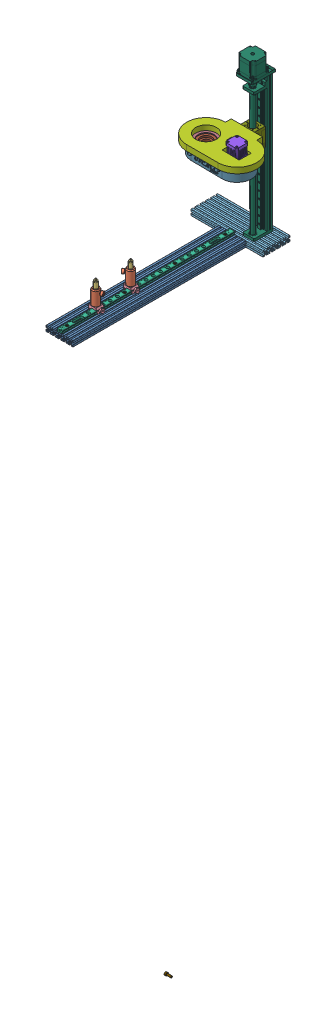
SolidWorks assembly OpenCALAssembly.v3.2, configuration Default. Lengths in mm.
Overall size (733.87 2470.14 969.59).
44 component instances, 19 part files, 57 mates.
Components (placement in the parent):
- 20-2020-Black-25-CL.stp-1: 20-2020-Black-25-CL.stp [Default] at (5.4558 13.0651 39.4201) size (94 20 600)
- PH50_M-Solidworks-1: PH50_M-Solidworks [Default] at (39.4918 57.7304 -95.7663) x (-0.331511 0 -0.943451) z (0.943451 0 -0.331511) size (25 50.44 35.14)
- TR75_M-Solidworks-1: TR75_M-Solidworks [Default] at (34.6119 36.3776 -93.7876) x (0.8365 0 0.547967) z (-0.547967 0 0.8365) size (12.67 80.02 12.87)
- RC1-Solidworks-1: RC1-Solidworks [Default] at (53.5095 23.0651 -81.0876) x (0 0 -1) z (1 0 0) size (25.4 16.53 39.23)
- 20-2020-Black-25-CLShort.stp-1: 20-2020-Black-25-CLShort.stp [Default] at (148.2574 13.0651 -570.5799) x (0 0 -1) z (1 0 0) size (94 20 250)
- PH50_M-Solidworks-2: PH50_M-Solidworks [Default] at (30.7203 57.7304 -211.3859) x (0.637938 0 0.770088) z (-0.770088 0 0.637938) size (25 50.44 35.14)
- TR75_M-Solidworks-2: TR75_M-Solidworks [Default] at (34.6119 34.7631 -214.9333) x (0.31409 0 0.949393) z (-0.949393 0 0.31409) size (12.67 80.02 12.87)
- RC1-Solidworks-2: RC1-Solidworks [Default] at (53.5095 23.0651 -202.2333) x (0 0 -1) z (1 0 0) size (25.4 16.53 39.23)
- RLA600_M-Solidworks-1: RLA600_M-Solidworks [Default] at (42.6639 28.1451 -260.6859) size (19.05 9.53 600)
- OpenCAL Assembly v3.2-1: OpenCAL Assembly v3.2 [Default] at (166.2971 1597.2966 -1408.9239) x (0.015214 0.027547 -0.999505) z (-0.999013 0.042148 -0.014045) size (158.86 120.73 246.6)
  - RotationStage-1: RotationStage [Default] at (-945.6056 1214.5248 22.5457) x (0.99962 0.027547 -0.000581) z (-0.000581 0.042148 0.999111) size (156.58 80 243.35)
  - Stepper with GT2 Pulley and Closed-Loop Belt-1: Stepper with GT2 Pulley and Closed-Loop Belt [Default] at (-980.4903 1273.0893 61.9746) x (-0.000908 0.042139 0.999111) z (0.99962 0.02756 -0.000254) size (166.51 64.5 74)
    - Copy of Assem2^Stepper with GT2 Pulley and Closed-Loop Belt-1: Copy of Assem2^Stepper with GT2 Pulley and Closed-Loop Belt [Default] at origin size (47.8 64.5 42.3) (virtual)
      - Nema17-1: Nema17 [Predeterminado] at (-104.7481 84.323 13.4322) x (0 0 1) z (1 0 0) size (42.3 64.5 47.8)
      - T5 Pulley-1: T5 Pulley [Predeterminado] at (-104.7481 37.623 13.4322) x (0 -1 0) z (0 0 1) size (14.8 16 16)
    - Belt-1: Belt [Default] at (-108.6865 25.623 13.493) size (153.36 6 74)
  - Collet with Gear and Toolholder-1: Collet with Gear and Toolholder [Default] at (-963.7475 1278.8086 52.0713) x (-0.99962 -0.027564 0.000171) z (-0.000991 0.042137 0.999111) size (98.27 60.66 98.27)
    - er32 x 34ths ToolHolderOpenCAL-1: er32 x 34ths ToolHolderOpenCAL [Default] at (-15.7823 32.6902 -13.7293) x (0.420729 0 0.907186) z (0.907186 0 -0.420729) size (74 44.7 74)
    - ER32 COLLET NUT-1: ER32 COLLET NUT [Default] at (3.8533 13.4515 11.5736) x (0 -1 0) z (0.99027 0 0.13916) size (22.61 50 50) (hidden)
    - ER32-20.step-1: ER32-20.step [Default] at (3.6132 -14.2638 13.2822) x (0.698361 0 0.715746) z (0 -1 0) size (32.96 32.96 40.01)
    - BallBearing-1: BallBearing [Default] at (3.6132 11.6902 13.2822) x (0.999353 0 0.035955) z (-0.035955 0 0.999353) size (72 9 72)
    - BallBearing-2: BallBearing [Default] at (3.6132 46.3902 13.2822) x (-0.871455 0 -0.490475) z (-0.490475 0 0.871455) size (72 9 72)
  - Rotation Stage Bottom Plate-1: Rotation Stage Bottom Plate [Default] at (-966.1754 1235.8663 67.174) x (0.00324 -0.042075 -0.999109) z (0.999615 0.027659 0.002077) size (210.36 36.77 134.78)
- ZStageAssm-2: ZStageAssm [Default] at (487.3353 488.304 -911.4771) x (0 -1 0) z (-1 0 0) size (562.65 93.47 86.84)
  - FSL40E350-BC-B57-1: FSL40E350-BC-B57 [Default] at (78.5613 293.4958 501.3397) size (562.65 93.47 86.84)
  - ZCarriage-1: ZCarriage [Default] at (-181.088 293.4958 501.3397) size (67.97 49.14 48.01)
- T-Nut 20 M5 v1.step-1: T-Nut 20 M5 v1.step [Default] at (42.6639 23.0651 14.3141) x (0 0 1) z (-1 0 0) size (10 4.5 9.24)
- socket head cap screw_am1-19: socket head cap screw_am1 [B18.3.1M - 5 x 0.8 x 8 Hex SHCS -- 8NHX] at (42.6639 30.6051 14.3141) x (0 -1 0) z (0 0 1) size (13 8.5 8.5)
- socket head cap screw_am1-20: socket head cap screw_am1 [B18.3.1M - 5 x 0.8 x 8 Hex SHCS -- 8NHX] at (42.6639 30.6051 -535.6859) x (0 -1 0) z (0 0 1) size (13 8.5 8.5)
- socket head cap screw_am1-21: socket head cap screw_am1 [B18.3.1M - 5 x 0.8 x 8 Hex SHCS -- 8NHX] at (42.6639 30.6051 -360.6859) x (0 -1 0) z (0 0 1) size (13 8.5 8.5)
- socket head cap screw_am1-22: socket head cap screw_am1 [B18.3.1M - 5 x 0.8 x 8 Hex SHCS -- 8NHX] at (42.6639 30.6051 -185.6859) x (0 -1 0) z (0 0 1) size (13 8.5 8.5)
- socket head cap screw_am1-23: socket head cap screw_am1 [B18.3.1M - 3 x 0.5 x 10 Hex SHCS -- 10NHX] at (156.5338 336.2143 -461.8522) x (0 1 0) z (0 0 1) size (13 5.5 5.5)
- socket head cap screw_am1-24: socket head cap screw_am1 [B18.3.1M - 3 x 0.5 x 10 Hex SHCS -- 10NHX] at (156.9774 336.2143 -492.8491) x (0 1 0) z (0 0 1) size (13 5.5 5.5)
- socket head cap screw_am1-25: socket head cap screw_am1 [B18.3.1M - 3 x 0.5 x 10 Hex SHCS -- 10NHX] at (125.9806 336.2143 -493.2927) x (0 1 0) z (0 0 1) size (13 5.5 5.5)
- socket head cap screw_am1-26: socket head cap screw_am1 [B18.3.1M - 3 x 0.5 x 10 Hex SHCS -- 10NHX] at (125.5369 336.2143 -462.2959) x (0 1 0) z (0 0 1) size (13 5.5 5.5)
- socket head cap screw_am1-27: socket head cap screw_am1 [B18.3.1M - 6 x 1.0 x 20 Hex SHCS -- 20NHX] at (97.1413 316.7143 -546.4733) x (0 0 -1) z (1 0 0) size (26 10 10)
- socket head cap screw_am1-28: socket head cap screw_am1 [B18.3.1M - 6 x 1.0 x 20 Hex SHCS -- 20NHX] at (77.1413 316.7143 -546.4733) x (0 0 -1) z (1 0 0) size (26 10 10)
- socket head cap screw_am1-29: socket head cap screw_am1 [B18.3.1M - 6 x 1.0 x 20 Hex SHCS -- 20NHX] at (97.1413 331.7143 -546.4733) x (0 0 -1) z (1 0 0) size (26 10 10)
- socket head cap screw_am1-30: socket head cap screw_am1 [B18.3.1M - 6 x 1.0 x 20 Hex SHCS -- 20NHX] at (77.1413 331.7143 -546.4733) x (0 0 -1) z (1 0 0) size (26 10 10)
- socket head cap screw_am1-31: socket head cap screw_am1 [B18.3.1M - 6 x 1.0 x 16 Hex SHCS -- 16NHX] at (316.7296 -1814.5075 -53.5357) size (22 10 10)
- socket head cap screw_am1-32: socket head cap screw_am1 [B18.3.1M - 6 x 1.0 x 16 Hex SHCS -- 16NHX] at (135.3565 328.2143 -537.5447) x (0 1 0) z (0 0 1) size (22 10 10)
- socket head cap screw_am1-33: socket head cap screw_am1 [B18.3.1M - 6 x 1.0 x 16 Hex SHCS -- 16NHX] at (37.4816 328.2143 -420.4078) x (0 1 0) z (0 0 1) size (22 10 10)
- socket head cap screw_am1-34: socket head cap screw_am1 [B18.3.1M - 6 x 1.0 x 16 Hex SHCS -- 16NHX] at (38.9942 328.2143 -537.4009) x (0 1 0) z (0 0 1) size (22 10 10)
- socket head cap screw_am1-35: socket head cap screw_am1 [B18.3.1M - 6 x 1.0 x 16 Hex SHCS -- 16NHX] at (135.4097 328.2143 -420.3812) x (0 1 0) z (0 0 1) size (22 10 10)
Mates (geometry in assembly coordinates):
- Concentric1: concentric aligned: circle of PH50_M-Solidworks-1; cylinder of TR75_M-Solidworks-1 through (34.6119 111.3838 -93.7876) axis (0 1 0) radius 6.3373
- Concentric2: concentric anti-aligned: circle of PH50_M-Solidworks-1; circle of RC1-Solidworks-1
- Coincident4: coincident anti-aligned: plane of PH50_M-Solidworks-1 through (43.7754 38.5591 -67.7092) normal (0 -1 0); plane of RC1-Solidworks-1 through (21.9119 38.5591 -81.0876) normal (0 1 0)
- Parallel1: parallel aligned: plane of 20-2020-Black-25-CL.stp-1 through (-3.0442 4.5651 39.4201) normal (0 0 1); plane of RC1-Solidworks-1 through (21.9119 23.0651 -81.0876) normal (0 0 1)
- Coincident6: coincident aligned: line of 20-2020-Black-25-CL.stp-1 through (45.5938 23.0651 -560.5799) axis (0 0 1); line of RC1-Solidworks-1 through (45.5938 23.0651 -106.4876) axis (0 0 1)
- Coincident7: coincident anti-aligned: plane of 20-2020-Black-25-CL.stp-1 through (32.4558 23.0651 14.4201) normal (0 1 0); plane of RC1-Solidworks-1 through (21.9119 23.0651 -81.0876) normal (0 -1 0)
- Coincident13: coincident anti-aligned: plane of 20-2020-Black-25-CL.stp-1 through (89.4558 4.5651 14.4201) normal (1 0 0); plane of 20-2020-Black-25-CL.stp-3 through (89.4558 13.0651 -350.9237) normal (-1 0 0)
- Concentric3: concentric aligned: circle of PH50_M-Solidworks-2; cylinder of TR75_M-Solidworks-2 through (34.6119 109.7693 -214.9333) axis (0 1 0) radius 6.3373
- Concentric4: concentric anti-aligned: circle of PH50_M-Solidworks-2; circle of RC1-Solidworks-2
- Coincident21: coincident anti-aligned: plane of PH50_M-Solidworks-2 through (16.9784 38.5591 -236.2196) normal (0 -1 0); plane of RC1-Solidworks-2 through (21.9119 38.5591 -202.2333) normal (0 1 0)
- Parallel2: parallel aligned: plane of 20-2020-Black-25-CL.stp-1 through (-3.0442 4.5651 39.4201) normal (0 0 1); plane of RC1-Solidworks-2 through (21.9119 23.0651 -202.2333) normal (0 0 1)
- Coincident22: coincident aligned: line of 20-2020-Black-25-CL.stp-1 through (45.5938 23.0651 -560.5799) axis (0 0 1); line of RC1-Solidworks-2 through (45.5938 23.0651 -227.6333) axis (0 0 1)
- Coincident23: coincident anti-aligned: plane of 20-2020-Black-25-CL.stp-1 through (32.4558 23.0651 14.4201) normal (0 1 0); plane of RC1-Solidworks-2 through (21.9119 23.0651 -202.2333) normal (0 -1 0)
- Parallel4: parallel anti-aligned: line of 20-2020-Black-25-CL.stp-1 through (50.9558 23.0651 39.4201) axis (-1 0 0); line of RLA600_M-Solidworks-1 through (36.3393 23.3191 39.3141) axis (1 0 0)
- Coincident28: coincident anti-aligned: plane of 20-2020-Black-25-CL.stp-1 through (50.9558 23.0651 14.4201) normal (0 1 0); plane of RLA600_M-Solidworks-1 through (52.1889 23.0651 39.3141) normal (0 -1 0)
- Coincident34: coincident aligned: plane of 20-2020-Black-25-CL.stp-1 through (57.8178 23.0651 14.4201) normal (0 1 0); plane of 20-2020-Black-25-CLShort.stp-1 through (123.2574 23.0651 -567.4419) normal (0 1 0)
- Coincident35: coincident anti-aligned: plane of 20-2020-Black-25-CL.stp-1 through (5.4558 13.0651 -560.5799) normal (0 0 -1); plane of 20-2020-Black-25-CLShort.stp-1 through (123.2574 21.5651 -560.5799) normal (0 0 1)
- Coincident36: coincident anti-aligned: plane of 20-2020-Black-25-CLShort.stp-1 through (123.2574 23.0651 -641.4419) normal (0 1 0); plane of ZStageAssm-2/FSL40E350-BC-B57-1 through (87.1413 23.0651 -604.1733) normal (0 -1 0)
- Parallel5: parallel aligned: plane of 20-2020-Black-25-CLShort.stp-1 through (148.2574 4.5651 -562.0799) normal (1 0 0); plane of ZStageAssm-2/FSL40E350-BC-B57-1 through (107.1413 23.0651 -636.6733) normal (1 0 0)
- Concentric13: concentric anti-aligned: circle of OpenCAL Assembly v3.2-1/RotationStage-1; cylinder of ZStageAssm-2/ZCarriage-1 through (97.1413 316.7143 -566.4733) axis (0 0 1) radius 3
- Parallel8: parallel anti-aligned: plane of OpenCAL Assembly v3.2-1/RotationStage-1 through (141.2662 359.2143 -566.4733) normal (1 0 0); plane of ZStageAssm-2/ZCarriage-1 through (111.1412 291.7143 -586.5733) normal (-1 0 0)
- Coincident42: coincident aligned: plane of OpenCAL Assembly v3.2-1/RotationStage-1 through (78.6927 359.2143 -566.4733) normal (0 0 -1); plane of ZStageAssm-2/ZCarriage-1 through (111.1413 356.7143 -566.4733) normal (0 0 -1)
- Concentric14: concentric aligned: cylinder of OpenCAL Assembly v3.2-1/Rotation Stage Bottom Plate-1 through (135.3565 329.2143 -537.5447) axis (0 -1 0) radius 2.9; cylinder of socket head cap screw_am-3 through (135.3565 296.4643 -537.5447) axis (0 -1 0) radius 5
- Coincident43: coincident anti-aligned: plane of OpenCAL Assembly v3.2-1/Rotation Stage Bottom Plate-1 through (133.3356 334.2143 -539.6246) normal (0 -1 0); plane of socket head cap screw_am-3 through (130.3565 334.2143 -537.5447) normal (0 1 0)
- Concentric15: concentric aligned: cylinder of OpenCAL Assembly v3.2-1/Rotation Stage Bottom Plate-1 through (37.4816 329.2143 -420.4078) axis (0 -1 0) radius 5; cylinder of socket head cap screw_am-4 through (37.4816 296.4643 -420.4078) axis (0 -1 0) radius 5
- Coincident44: coincident anti-aligned: plane of OpenCAL Assembly v3.2-1/Rotation Stage Bottom Plate-1 through (35.4607 334.2143 -422.4877) normal (0 -1 0); plane of socket head cap screw_am-4 through (32.4816 334.2143 -420.4078) normal (0 1 0)
- Concentric16: concentric aligned: cylinder of OpenCAL Assembly v3.2-1/Rotation Stage Bottom Plate-1 through (38.9942 329.2143 -537.4009) axis (0 -1 0) radius 2.9; cylinder of socket head cap screw_am-5 through (38.9942 296.4643 -537.4009) axis (0 -1 0) radius 5
- Coincident45: coincident anti-aligned: plane of OpenCAL Assembly v3.2-1/Rotation Stage Bottom Plate-1 through (36.9733 334.2143 -539.4808) normal (0 -1 0); plane of socket head cap screw_am-5 through (33.9942 334.2143 -537.4009) normal (0 1 0)
- Concentric17: concentric: cylinder of OpenCAL Assembly v3.2-1/Rotation Stage Bottom Plate-1 through (135.4097 329.2143 -420.3812) axis (0 -1 0) radius 2.9; cylinder of socket head cap screw_am-6 through (135.4097 296.4643 -420.3812) axis (0 -1 0) radius 5
- Coincident46: coincident: plane of OpenCAL Assembly v3.2-1/Rotation Stage Bottom Plate-1 through (135.4147 334.2143 -423.2812) normal (0 -1 0); plane of socket head cap screw_am-6 through (130.4097 334.2143 -420.3812) normal (0 1 0)
- Concentric22: concentric aligned: cylinder of OpenCAL Assembly v3.2-1/RotationStage-1 through (97.1413 316.7143 -546.4733) axis (0 0 1) radius 5.5; cylinder of socket head cap screw_am-11 through (97.1413 316.7143 -514.7233) axis (0 0 1) radius 5
- Coincident51: coincident anti-aligned: plane of OpenCAL Assembly v3.2-1/RotationStage-1 through (94.5651 314.3451 -552.4733) normal (0 0 1); plane of socket head cap screw_am-11 through (97.1413 321.7143 -552.4733) normal (0 0 -1)
- Concentric23: concentric aligned: cylinder of OpenCAL Assembly v3.2-1/RotationStage-1 through (77.1413 316.7143 -546.4733) axis (0 0 1) radius 3.5; cylinder of socket head cap screw_am-12 through (77.1413 316.7143 -514.7233) axis (0 0 1) radius 5
- Coincident52: coincident anti-aligned: plane of OpenCAL Assembly v3.2-1/RotationStage-1 through (74.5651 314.3451 -552.4733) normal (0 0 1); plane of socket head cap screw_am-12 through (77.1413 321.7143 -552.4733) normal (0 0 -1)
- Concentric24: concentric aligned: cylinder of OpenCAL Assembly v3.2-1/RotationStage-1 through (97.1413 331.7143 -546.4733) axis (0 0 1) radius 3.5; cylinder of socket head cap screw_am-13 through (97.1413 331.7143 -514.7233) axis (0 0 1) radius 5
- Coincident53: coincident anti-aligned: plane of OpenCAL Assembly v3.2-1/RotationStage-1 through (94.5651 329.3451 -552.4733) normal (0 0 1); plane of socket head cap screw_am-13 through (97.1413 336.7143 -552.4733) normal (0 0 -1)
- Concentric25: concentric aligned: cylinder of OpenCAL Assembly v3.2-1/RotationStage-1 through (77.1413 331.7143 -546.4733) axis (0 0 1) radius 3.5; cylinder of socket head cap screw_am-14 through (77.1413 331.7143 -514.7233) axis (0 0 1) radius 5
- Coincident54: coincident anti-aligned: plane of OpenCAL Assembly v3.2-1/RotationStage-1 through (74.5651 329.3451 -552.4733) normal (0 0 1); plane of socket head cap screw_am-14 through (77.1413 336.7143 -552.4733) normal (0 0 -1)
- Concentric26: concentric anti-aligned: cylinder of OpenCAL Assembly v3.2-1/Stepper with GT2 Pulley and Closed-Loop Belt-1/Copy of Assem2^Stepper with GT2 Pulley and Closed-Loop Belt-1/Nema17-1 through (156.5338 388.748 -461.8522) axis (0 1 0) radius 1.6; cylinder of socket head cap screw_am-15 through (156.5338 304.4643 -461.8522) axis (0 -1 0) radius 2.75
- Coincident55: coincident anti-aligned: plane of OpenCAL Assembly v3.2-1/RotationStage-1 through (78.6927 339.2143 -498.3051) normal (0 -1 0); plane of socket head cap screw_am-15 through (153.7838 339.2143 -461.8522) normal (0 1 0)
- Concentric27: concentric anti-aligned: cylinder of OpenCAL Assembly v3.2-1/Stepper with GT2 Pulley and Closed-Loop Belt-1/Copy of Assem2^Stepper with GT2 Pulley and Closed-Loop Belt-1/Nema17-1 through (156.9774 388.748 -492.8491) axis (0 1 0) radius 1.6; cylinder of socket head cap screw_am-16 through (156.9774 304.4643 -492.8491) axis (0 -1 0) radius 2.75
- Coincident56: coincident anti-aligned: plane of OpenCAL Assembly v3.2-1/RotationStage-1 through (78.6927 339.2143 -498.3051) normal (0 -1 0); plane of socket head cap screw_am-16 through (154.2274 339.2143 -492.8491) normal (0 1 0)
- Concentric28: concentric anti-aligned: cylinder of OpenCAL Assembly v3.2-1/Stepper with GT2 Pulley and Closed-Loop Belt-1/Copy of Assem2^Stepper with GT2 Pulley and Closed-Loop Belt-1/Nema17-1 through (125.9806 388.748 -493.2927) axis (0 1 0) radius 1.6; cylinder of socket head cap screw_am-17 through (125.9806 304.4643 -493.2927) axis (0 -1 0) radius 2.75
- Coincident57: coincident anti-aligned: plane of OpenCAL Assembly v3.2-1/RotationStage-1 through (78.6927 339.2143 -498.3051) normal (0 -1 0); plane of socket head cap screw_am-17 through (123.2306 339.2143 -493.2927) normal (0 1 0)
- Concentric29: concentric anti-aligned: cylinder of OpenCAL Assembly v3.2-1/Stepper with GT2 Pulley and Closed-Loop Belt-1/Copy of Assem2^Stepper with GT2 Pulley and Closed-Loop Belt-1/Nema17-1 through (125.5369 388.748 -462.2959) axis (0 1 0) radius 1.6; cylinder of socket head cap screw_am-18 through (125.5369 304.4643 -462.2959) axis (0 -1 0) radius 2.75
- Coincident58: coincident anti-aligned: plane of OpenCAL Assembly v3.2-1/RotationStage-1 through (78.6927 339.2143 -498.3051) normal (0 -1 0); plane of socket head cap screw_am-18 through (122.7869 339.2143 -462.2959) normal (0 1 0)
- Concentric30: concentric aligned: cylinder of RLA600_M-Solidworks-1 through (42.6639 32.3361 14.3141) axis (0 1 0) radius 3.3655; cylinder of socket head cap screw_am-19 through (42.6639 62.3551 14.3141) axis (0 1 0) radius 4.25
- Coincident59: coincident anti-aligned: plane of RLA600_M-Solidworks-1 through (46.0294 25.6051 14.3141) normal (0 1 0); plane of socket head cap screw_am-19 through (46.9139 25.6051 14.3141) normal (0 -1 0)
- Concentric31: concentric aligned: cylinder of RLA600_M-Solidworks-1 through (42.6639 32.3361 -535.6859) axis (0 1 0) radius 3.3655; cylinder of socket head cap screw_am-20 through (42.6639 62.3551 -535.6859) axis (0 1 0) radius 4.25
- Coincident60: coincident anti-aligned: plane of RLA600_M-Solidworks-1 through (46.0294 25.6051 -535.6859) normal (0 1 0); plane of socket head cap screw_am-20 through (46.9139 25.6051 -535.6859) normal (0 -1 0)
- Concentric32: concentric aligned: cylinder of RLA600_M-Solidworks-1 through (42.6639 32.3361 -360.6859) axis (0 1 0) radius 3.3655; cylinder of socket head cap screw_am-21 through (42.6639 62.3551 -360.6859) axis (0 1 0) radius 4.25
- Coincident61: coincident anti-aligned: plane of RLA600_M-Solidworks-1 through (46.0294 25.6051 -360.6859) normal (0 1 0); plane of socket head cap screw_am-21 through (46.9139 25.6051 -360.6859) normal (0 -1 0)
- Concentric33: concentric aligned: cylinder of RLA600_M-Solidworks-1 through (42.6639 32.3361 -185.6859) axis (0 1 0) radius 3.3655; cylinder of socket head cap screw_am-22 through (42.6639 62.3551 -185.6859) axis (0 1 0) radius 4.25
- Coincident62: coincident anti-aligned: plane of RLA600_M-Solidworks-1 through (46.0294 25.6051 -185.6859) normal (0 1 0); plane of socket head cap screw_am-22 through (46.9139 25.6051 -185.6859) normal (0 -1 0)
- Concentric34: concentric anti-aligned: cylinder of socket head cap screw_am-19 through (42.6639 62.3551 14.3141) axis (0 1 0) radius 2.5; circle of T-Nut 20 M5 v1.step-1
- Parallel9: parallel: line of 20-2020-Black-25-CL.stp-1 through (48.4508 20.3313 -560.5799) axis (0 0 1); plane of T-Nut 20 M5 v1.step-1 through (39.6639 22.9651 14.3141) normal (-1 0 0)
- Coincident64: coincident anti-aligned: plane of 20-2020-Black-25-CL.stp-1 through (36.9688 21.5651 14.4201) normal (0 -1 0); plane of T-Nut 20 M5 v1.step-1 through (39.6639 21.5651 14.3141) normal (0 1 0)
